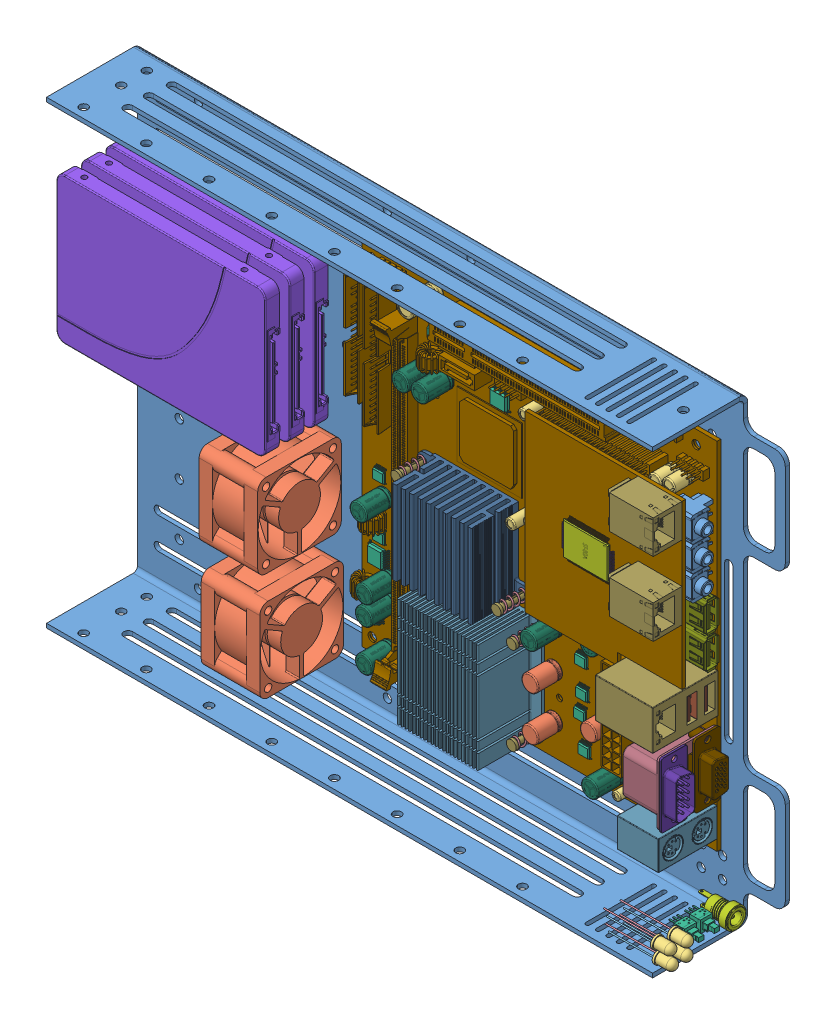
SolidWorks assembly kubebox_tray_itx, configuration Predeterminado. Lengths in mm.
Overall size (310 220 48.86).
125 component instances, 32 part files, 1 mates.
Components (placement in the parent):
- kubebox_tray-1: kubebox_tray [Predeterminado] at (-106.1016 -89.1854 250) size (310 220 45.5)
- Fan-40x40-1: Fan-40x40 [28mm] at (-84.3442 -51.7342 270.7277) x (0 0 -1) z (-1 0 0) size (48.86 43.8 28.03)
- LED 5mm green.step-2: LED 5mm green.step [Predeterminado] at (111.4078 -83.8857 281.3681) x (-0.004686 -0.000144 -0.999989) z (0.999988 0.001702 -0.004686) size (5.8 5.4 33.7)
  - F6rper 5mm.step-1: F6rper 5mm.step [Predeterminado] at origin size (5.8 5.4 8.7)
  - Anode.step-1: Anode.step [Predeterminado] at (0 1.27 -25) size (0.54 0.54 25)
  - Kadode.step-1: Kadode.step [Predeterminado] at (0 -1.27 -25) size (0.54 0.54 23.5)
- LED 5mm green.step-3: LED 5mm green.step [Predeterminado] at (111.773 -77.6908 281.5141) x (-0.004686 -0.000144 -0.999989) z (0.999988 0.001702 -0.004686) size (5.8 5.4 33.7)
  - F6rper 5mm.step-1: F6rper 5mm.step [Predeterminado] at origin size (5.8 5.4 8.7)
  - Anode.step-1: Anode.step [Predeterminado] at (0 1.27 -25) size (0.54 0.54 25)
  - Kadode.step-1: Kadode.step [Predeterminado] at (0 -1.27 -25) size (0.54 0.54 23.5)
- LED 5mm green.step-4: LED 5mm green.step [Predeterminado] at (111.6884 -83.9214 288.5994) x (-0.004686 -0.000144 -0.999989) z (0.999988 0.001702 -0.004686) size (5.8 5.4 33.7)
  - F6rper 5mm.step-1: F6rper 5mm.step [Predeterminado] at origin size (5.8 5.4 8.7)
  - Anode.step-1: Anode.step [Predeterminado] at (0 1.27 -25) size (0.54 0.54 25)
  - Kadode.step-1: Kadode.step [Predeterminado] at (0 -1.27 -25) size (0.54 0.54 23.5)
- LED 5mm green.step-5: LED 5mm green.step [Predeterminado] at (111.1 -77.7464 288.8261) x (-0.004686 -0.000144 -0.999989) z (0.999988 0.001702 -0.004686) size (5.8 5.4 33.7)
  - F6rper 5mm.step-1: F6rper 5mm.step [Predeterminado] at origin size (5.8 5.4 8.7)
  - Anode.step-1: Anode.step [Predeterminado] at (0 1.27 -25) size (0.54 0.54 25)
  - Kadode.step-1: Kadode.step [Predeterminado] at (0 -1.27 -25) size (0.54 0.54 23.5)
- Toggle Button (6 x 6 x 10mm) - NON Latching.stp-1: Toggle Button (6 x 6 x 10mm) - NON Latching.stp [Predeterminado] at (107.7716 -80.5751 266.7149) x (0 1 0) z (1 0 0) size (5.74 5.82 13.39)
- Toggle Button (6 x 6 x 10mm) - NON Latching.stp-2: Toggle Button (6 x 6 x 10mm) - NON Latching.stp [Predeterminado] at (107.7786 -80.552 274.244) x (0 1 0) z (1 0 0) size (5.74 5.82 13.39)
- Fan-40x40-2: Fan-40x40 [28mm] at (-85.3503 -0.9212 270.7277) x (0 0 -1) z (-1 0 0) size (48.86 43.8 28.03)
- 2.1mm x 5.5mm Round Chasis Female Socket DC Connector Jack-1: 2.1mm x 5.5mm Round Chasis Female Socket DC Connector Jack [Default] at (113.9605 -80.8969 257.09) x (0 0 -1) z (1 0 0) size (10 10 17.7)
- Standard 520 model-1: Standard 520 model [Default] at (-125.8554 63.2761 262.1971) x (0 1 0) z (1 0 0) size (69.85 7 100.3)
- Standard 520 model-2: Standard 520 model [Default] at (-125.8457 63.2851 273.7903) x (0 1 0) z (1 0 0) size (69.85 7 100.3)
- Standard 520 model-3: Standard 520 model [Default] at (-125.8434 63.2833 285.5347) x (0 1 0) z (1 0 0) size (69.85 7 100.3)
- Motherboard-1: Motherboard [Default] at (24.0384 27.9346 255.9838) x (0 1 0) z (1 0 0) size (170 37.23 177.79)
  - Motherboard-Mini-ITX-1: Motherboard-Mini-ITX [Default] at origin size (170 18.6 170)
  - User Library-TS-65259-ZH-1: User Library-TS-65259-ZH [Default] at (-7.4545 1.8 -30) x (0 0 -1) z (1 0 0) size (54 24.6 40.05)
    - User Library-TS-65259-ZH_BGA Heat Sink-2: User Library-TS-65259-ZH_BGA Heat Sink [Default] at origin size (54 22.5 40.05)
    - User Library-TS-65259-ZH_T710 Material-1: User Library-TS-65259-ZH_T710 Material [Default] x (1 0 0) z (0 -1 0) size (31.75 31.75 0.2)
    - User Library-TS-65259-ZH_Brass Pin-1: User Library-TS-65259-ZH_Brass Pin [Default] at (-24 14.77 -15.7) size (4.7 16.87 4.7)
    - User Library-TS-65259-ZH_Spring-Uncompressed-1: User Library-TS-65259-ZH_Spring-Uncompressed [Default] at (-24 14.3143 -15.7) x (1 0 0) z (0 -1 0) size (5.34 6 13)
    - User Library-TS-65259-ZH_Brass Pin-2: User Library-TS-65259-ZH_Brass Pin [Default] at (24 14.77 15.7) size (4.7 16.87 4.7)
    - User Library-TS-65259-ZH_Spring-Uncompressed-2: User Library-TS-65259-ZH_Spring-Uncompressed [Default] at (24 0.7057 15.7) x (1 0 0) z (0 1 0) size (5.34 6 13)
  - Heat Sink A-1: Heat Sink A [Default] at (-56.3 1.8 -22.5) x (0 0 -1) z (1 0 0) size (50 26.5 52)
  - User Library-TS-65259-ZH_Brass Pin-1: User Library-TS-65259-ZH_Brass Pin [Default] at (-35.3 14.77 -44.5) x (0 0 -1) z (1 0 0) size (4.7 16.87 4.7)
  - User Library-TS-65259-ZH_Spring-Uncompressed-1: User Library-TS-65259-ZH_Spring-Uncompressed [Default] at (-35.3 0.8156 -44.5) x (0.439893 0 -0.89805) z (0 1 0) size (5.34 6 13)
  - User Library-CAPACITOR-2-1: User Library-CAPACITOR-2 [D=8] at (-79.4531 -4.5974 -71.4991) size (8.26 14.29 8.25)
  - User Library-CAPACITOR-2-2: User Library-CAPACITOR-2 [D=8] at (-50.3757 -4.5974 -71.4991) size (8.26 14.29 8.25)
  - User Library-CAPACITOR-2-3: User Library-CAPACITOR-2 [D=8] at (-17.5304 -4.5974 -74.0227) size (8.26 14.29 8.25)
  - User Library-CAPACITOR-2-4: User Library-CAPACITOR-2 [D=8] at (-59.6152 -4.5974 -71.4991) size (8.26 14.29 8.25)
  - User Library-CAPACITOR-2-5: User Library-CAPACITOR-2 [D=8] at (46.2267 -4.5974 -44.8893) x (-0.064546 0 -0.997915) z (0.997915 0 -0.064546) size (8.26 14.29 8.25)
  - User Library-CAPACITOR-2-6: User Library-CAPACITOR-2 [D=8] at (46.2268 -4.5974 -54.0316) size (8.26 14.29 8.25)
  - User Library-CAPACITOR-2-7: User Library-CAPACITOR-2 [D=8] at (-18.1774 -4.5974 36.0078) x (-0.064546 0 -0.997915) z (0.997915 0 -0.064546) size (8.26 14.29 8.25)
  - User Library-CAPACITOR-2-8: User Library-CAPACITOR-2 [D=8] at (9.1349 -4.5974 42.427) x (-0.064546 0 -0.997915) z (0.997915 0 -0.064546) size (8.26 14.29 8.25)
  - User Library-CAPACITOR-2-9: User Library-CAPACITOR-2 [D=8] at (53.4161 -4.5974 31.2418) x (-0.064546 0 -0.997915) z (0.997915 0 -0.064546) size (8.26 14.29 8.25)
  - User Library-CAPACITOR-2-10: User Library-CAPACITOR-2 [D=8] at (27.2615 -4.5974 57.1967) x (-0.064546 0 -0.997915) z (0.997915 0 -0.064546) size (8.26 14.29 8.25)
  - User Library-CAPACITOR-2-11: User Library-CAPACITOR-2 [D=8] at (17.5542 -4.5974 22.737) x (-0.064546 0 -0.997915) z (0.997915 0 -0.064546) size (8.26 14.29 8.25)
  - User Library-CAPACITOR-2-12: User Library-CAPACITOR-2 [D=8] at (-76.824 -4.5974 36.7263) x (-0.064546 0 -0.997915) z (0.997915 0 -0.064546) size (8.26 14.29 8.25)
  - User Library-USB Socket-1: User Library-USB Socket [Default] at (14.3 1.8 78.48) size (14.6 8.03 14.23)
  - User Library-USB Socket-2: User Library-USB Socket [Default] at (-1.1 1.8 78.48) size (14.6 8.03 14.23)
  - User Library-DB15HD-1: User Library-DB15HD [Predeterminado] at (-47.5 23.6419 85.4) size (31 12.5 18)
  - User Library-DB15recept_straight-1: User Library-DB15recept_straight [Default] at (-47.5 7.6681 86.3906) size (30.81 12.55 17.86)
  - CUI-SJ1-3545N-1: CUI-SJ1-3545N [Pink] at (54 9.8 88.5) x (0 0 1) z (0 1 0) size (15 12.2 16.5)
  - SW3DPS-ELECTROLITIC CAPACITOR RADIAL 8X12-DEFAULT-1: SW3DPS-ELECTROLITIC CAPACITOR RADIAL 8X12-DEFAULT [Default] at (-69.4896 1.8 7.3403) x (0.957319 0 0.289034) z (-0.289034 0 0.957319) size (8 14.5 8)
  - User Library-Capacitor Radial Electrolitic-1: User Library-Capacitor Radial Electrolitic [CAPPR350-800X1500] at (79.996 1.8 -49.5016) x (0.219712 0 -0.975565) z (0.975565 0 0.219712) size (8.01 17.73 8)
  - User Library-QFP-24P400X400LS050h120-1: User Library-QFP-24P400X400LS050h120 [Default] at (-16.4 2.9831 53.4) x (0 0 -1) z (0 1 0) size (10.8 10.8 2.16)
  - User Library-so14p865x390ll600ls127h155-1: User Library-so14p865x390ll600ls127h155 [1] at (16.7443 1.8 54.05) x (0 0 -1) z (0 1 0) size (6 6.07 1.55)
  - User Library-ssop16p500x440ls065h200-1: User Library-ssop16p500x440ls065h200 [Default] at (70.8 1.8 -47) x (1 0 0) z (0 1 0) size (6.4 5 2)
  - User Library-ST-80A-1: User Library-ST-80A [Default] at (2.5646 1.3604 55.1237) size (15.56 1.47 21.26)
    - User Library-ST-80A_ST-80A_Body-1: User Library-ST-80A_ST-80A_Body [Default] at (1.4361 0.5396 -1.1244) size (12 1.4 12)
    - User Library-ST-80A_Pin-9: User Library-ST-80A_Pin [1] at (-3.4851 0.946 5.8923) x (0 0 1) z (-1 0 0) size (1.78 0.97 9.91)
    - User Library-ST-80A_Pin1-9: User Library-ST-80A_Pin1 [Default] at (8.4529 0.946 4.2147) size (1.78 0.97 19.05)
    - User Library-ST-80A_Pin1-10: User Library-ST-80A_Pin1 [Default] at (-5.5806 0.946 -14.3781) x (-1 0 0) z (0 0 -1) size (1.78 0.97 19.05)
    - User Library-ST-80A_Pin-11: User Library-ST-80A_Pin [1] at (5.9383 0.946 -8.1412) x (0 0 -1) z (1 0 0) size (1.78 0.97 9.91)
    - User Library-ST-80A_Pin-12: User Library-ST-80A_Pin [1] at (-5.5806 0.946 -6.296) x (-1 0 0) z (0 0 -1) size (1.78 0.97 9.91)
    - User Library-ST-80A_Pin-13: User Library-ST-80A_Pin [1] at (8.4529 0.946 3.1528) size (1.78 0.97 9.91)
  - User Library-tsop24p600x1640ls050h120-1: User Library-tsop24p600x1640ls050h120 [Default] at (-11 2 14.8) x (0 0 -1) z (0 1 0) size (18 6 1.2)
  - User Library-Capacitor Radial Electrolitic-2: User Library-Capacitor Radial Electrolitic [CAPPR200-500X1100] at (-43.7308 1.8 -20.0233) size (5.01 13.73 5)
  - User Library-ssop16p500x440ls065h200-2: User Library-ssop16p500x440ls065h200 [1] at (-42.25 2.3907 -76.2) x (0 0 1) z (0 1 0) size (9.6 7.5 3)
  - User Library-ST-80A-2: User Library-ST-80A [1] at (30.2619 1.2704 34.3205) size (19.16 1.47 25.16)
    - User Library-ST-80A_ST-80A_Body-1: User Library-ST-80A_ST-80A_Body [1] at (1.4361 0.5396 -1.1244) size (15.6 1.4 21.6)
    - User Library-ST-80A_Pin-9: User Library-ST-80A_Pin [1] at (-2.9793 0.946 10.6955) x (0 0 1) z (-1 0 0) size (1.78 0.97 9.91)
    - User Library-ST-80A_Pin1-9: User Library-ST-80A_Pin1 [Default] at (10.2541 0.946 8.6715) size (1.78 0.97 19.05)
    - User Library-ST-80A_Pin1-10: User Library-ST-80A_Pin1 [Default] at (-7.3799 0.946 -9.9213) x (-1 0 0) z (0 0 -1) size (1.78 0.97 19.05)
    - User Library-ST-80A_Pin-11: User Library-ST-80A_Pin [1] at (6.4695 0.946 -12.9392) x (0 0 -1) z (1 0 0) size (1.78 0.97 9.91)
    - User Library-ST-80A_Pin-12: User Library-ST-80A_Pin [1] at (-5.5806 0.946 -6.296) x (-1 0 0) z (0 0 -1) size (1.78 0.97 9.91)
    - User Library-ST-80A_Pin-13: User Library-ST-80A_Pin [1] at (8.4529 0.946 3.1528) size (1.78 0.97 9.91)
  - User Library-ssop16p500x440ls065h200-3: User Library-ssop16p500x440ls065h200 [Default] at (-36.8 2.4 61.5) x (1 0 0) z (0 1 0) size (6.4 5 2)
  - SW3DPS-ELECTROLITIC CAPACITOR RADIAL 8X12-DEFAULT-2: SW3DPS-ELECTROLITIC CAPACITOR RADIAL 8X12-DEFAULT [Default] at (-54.5523 1.8 35.2905) x (0.957319 0 0.289034) z (-0.289034 0 0.957319) size (8 14.5 8)
  - SW3DPS-ELECTROLITIC CAPACITOR RADIAL 8X12-DEFAULT-3: SW3DPS-ELECTROLITIC CAPACITOR RADIAL 8X12-DEFAULT [Default] at (-48.2292 1.8 7.3403) x (0.957319 0 0.289034) z (-0.289034 0 0.957319) size (8 14.5 8)
  - User Library-TS-65259-ZH_Brass Pin-2: User Library-TS-65259-ZH_Brass Pin [Default] at (-77.3 14.77 -44.5) x (0.837243 0 0.546832) z (-0.546832 0 0.837243) size (4.7 16.87 4.7)
  - User Library-TS-65259-ZH_Brass Pin-3: User Library-TS-65259-ZH_Brass Pin [Default] at (-77.3 14.77 -0.5) x (0 0 -1) z (1 0 0) size (4.7 16.87 4.7)
  - User Library-TS-65259-ZH_Brass Pin-4: User Library-TS-65259-ZH_Brass Pin [Default] at (-35.3 14.77 -0.5) x (0.837243 0 0.546832) z (-0.546832 0 0.837243) size (4.7 16.87 4.7)
  - User Library-TS-65259-ZH_Spring-Uncompressed-2: User Library-TS-65259-ZH_Spring-Uncompressed [Default] at (-35.3 0.8156 -0.5) x (-0.772723 0 0.634744) z (0 1 0) size (5.34 6 13)
  - User Library-TS-65259-ZH_Spring-Uncompressed-3: User Library-TS-65259-ZH_Spring-Uncompressed [Default] at (-77.3 0.8156 -44.5) x (0.999805 0 0.01976) z (0 1 0) size (5.34 6 13)
  - User Library-TS-65259-ZH_Spring-Uncompressed-4: User Library-TS-65259-ZH_Spring-Uncompressed [Default] at (-77.3 0.8156 -0.5) x (-0.998104 0 0.061542) z (0 1 0) size (5.34 6 13)
  - CUI-SJ1-3545N-2: CUI-SJ1-3545N [Green] at (41.8 9.8 88.5) x (0 0 1) z (0 1 0) size (15 12.2 16.5)
  - CUI-SJ1-3545N-3: CUI-SJ1-3545N [Blue] at (29.6 9.8 88.5) x (0 0 1) z (0 1 0) size (15 12.2 16.5)
  - User Library-Capacitor Radial Electrolitic-4: User Library-Capacitor Radial Electrolitic [CAPPR250-630X980] at (64.5347 1.81 71.4955) x (0.219712 0 -0.975565) z (0.975565 0 0.219712) size (6.31 12.53 6.3)
  - User Library-Capacitor Radial Electrolitic-5: User Library-Capacitor Radial Electrolitic [CAPPR250-630X1500] at (41.4632 1.81 58.7461) x (0.219712 0 -0.975565) z (0.975565 0 0.219712) size (6.31 17.73 6.3)
  - User Library-Capacitor Radial Electrolitic-6: User Library-Capacitor Radial Electrolitic [CAPPR200-500X1150] at (41.4632 1.81 52.1875) x (0.219712 0 -0.975565) z (0.975565 0 0.219712) size (5.01 14.23 5)
  - User Library-Capacitor Radial Electrolitic-7: User Library-Capacitor Radial Electrolitic [CAPPR250-630X980] at (63.1844 1.81 64.8938) x (0.219712 0 -0.975565) z (0.975565 0 0.219712) size (6.31 12.53 6.3)
  - Samtec-USB-A-D-S-B-VU-1: Samtec-USB-A-D-S-B-VU [Default] at (-19.2 2.9 76.495) size (15.8 19.67 17.65)
  - User Library-RJ45-8P-Pipe-Cat6-1: User Library-RJ45-8P-Pipe-Cat6 [Default] at (-19.2 18.4 64.2) size (21.35 33.02 27.5)
  - User Library-ssop16p500x440ls065h200-4: User Library-ssop16p500x440ls065h200 [Default] at (62.8 1.8 -49.5) x (1 0 0) z (0 1 0) size (6.4 5 2)
  - User Library-ssop16p500x440ls065h200-5: User Library-ssop16p500x440ls065h200 [Default] at (-49.8 2.6 22.5) x (1 0 0) z (0 1 0) size (6.4 5 2)
  - User Library-ssop16p500x440ls065h200-6: User Library-ssop16p500x440ls065h200 [Default] at (-72.8 2.6 23.5) x (1 0 0) z (0 1 0) size (6.4 5 2)
  - User Library-ssop16p500x440ls065h200-7: User Library-ssop16p500x440ls065h200 [Default] at (-36.3 2.6 22) x (1 0 0) z (0 1 0) size (6.4 5 2)
  - User Library-ssop16p500x440ls065h200-8: User Library-ssop16p500x440ls065h200 [Default] at (-58.8 2.6 21.5) x (1 0 0) z (0 1 0) size (6.4 5 2)
  - User Library-ssop16p500x440ls065h200-9: User Library-ssop16p500x440ls065h200 [Default] at (16.7 2.6 13) x (1 0 0) z (0 1 0) size (6.4 5 2)
  - User Library-so14p865x390ll600ls127h155-2: User Library-so14p865x390ll600ls127h155 [1] at (33.8028 1.8 55.0746) x (0 0 -1) z (0 1 0) size (6 6.07 1.55)
  - User Library-ssop16p500x440ls065h200-10: User Library-ssop16p500x440ls065h200 [Default] at (51.3 2.6 56.9) x (1 0 0) z (0 1 0) size (6.4 5 2)
  - User Library-ssop16p500x440ls065h200-11: User Library-ssop16p500x440ls065h200 [1] at (52.2 2.3907 -17.25) x (1 0 0) z (0 1 0) size (9.6 7.5 3)
  - User Library-ssop16p500x440ls065h200-12: User Library-ssop16p500x440ls065h200 [Default] at (-8.7786 1.8 -75.5) x (1 0 0) z (0 1 0) size (6.4 5 2)
  - User Library-ssop16p500x440ls065h200-13: User Library-ssop16p500x440ls065h200 [Default] at (-34.0566 1.8 -75.5) x (1 0 0) z (0 1 0) size (6.4 5 2)
  - User Library-ssop16p500x440ls065h200-14: User Library-ssop16p500x440ls065h200 [1] at (-66.75 2.3907 -79) x (0 0 1) z (0 1 0) size (9.6 7.5 3)
  - User Library-Capacitor Radial Electrolitic-8: User Library-Capacitor Radial Electrolitic [CAPPR200-500X1150] at (17.2298 1.81 6.0657) x (0.219712 0 -0.975565) z (0.975565 0 0.219712) size (5.01 14.23 5)
  - User Library-Capacitor Radial Electrolitic-9: User Library-Capacitor Radial Electrolitic [CAPPR200-500X1150] at (12.4626 1.81 -2.6529) x (0.219712 0 -0.975565) z (0.975565 0 0.219712) size (5.01 14.23 5)
  - User Library-CAPACITOR-2-13: User Library-CAPACITOR-2 [D=8] at (-30.2607 -4.5974 7.2973) x (-0.064546 0 -0.997915) z (0.997915 0 -0.064546) size (8.26 14.29 8.25)
  - User Library-Capacitor Radial Electrolitic-10: User Library-Capacitor Radial Electrolitic [CAPPR200-500X1150] at (60.8999 1.81 3.545) x (0.219712 0 -0.975565) z (0.975565 0 0.219712) size (5.01 14.23 5)
  - User Library-Capacitor Radial Electrolitic-11: User Library-Capacitor Radial Electrolitic [CAPPR150-400X700] at (7.4823 1.8 68.8681) x (0.219712 0 -0.975565) z (0.975565 0 0.219712) size (4.01 9.73 4)
  - User Library-Capacitor Radial Electrolitic-12: User Library-Capacitor Radial Electrolitic [CAPPR150-400X700] at (-79.4532 1.81 43.5549) x (0.219712 0 -0.975565) z (0.975565 0 0.219712) size (4.01 9.73 4)
  - Monitor connector Housing-1: Monitor connector Housing [Default] at (-47.5 23.6419 85.4) size (30.5 28.3 17.81)
  - User Library-ST-80A-3: User Library-ST-80A [1] at (24.7839 18.1404 41.3205) size (19.16 1.47 25.16)
    - User Library-ST-80A_ST-80A_Body-1: User Library-ST-80A_ST-80A_Body [1] at (1.4361 0.5396 -1.1244) size (15.6 1.4 21.6)
    - User Library-ST-80A_Pin-9: User Library-ST-80A_Pin [1] at (-2.9793 0.946 10.6955) x (0 0 1) z (-1 0 0) size (1.78 0.97 9.91)
    - User Library-ST-80A_Pin1-9: User Library-ST-80A_Pin1 [Default] at (10.2541 0.946 8.6715) size (1.78 0.97 19.05)
    - User Library-ST-80A_Pin1-10: User Library-ST-80A_Pin1 [Default] at (-7.3799 0.946 -9.9213) x (-1 0 0) z (0 0 -1) size (1.78 0.97 19.05)
    - User Library-ST-80A_Pin-11: User Library-ST-80A_Pin [1] at (6.4695 0.946 -12.9392) x (0 0 -1) z (1 0 0) size (1.78 0.97 9.91)
    - User Library-ST-80A_Pin-12: User Library-ST-80A_Pin [1] at (-5.5806 0.946 -6.296) x (-1 0 0) z (0 0 -1) size (1.78 0.97 9.91)
    - User Library-ST-80A_Pin-13: User Library-ST-80A_Pin [1] at (8.4529 0.946 3.1528) size (1.78 0.97 9.91)
  - User Library-RJ45-8P-Pipe-Cat6-2: User Library-RJ45-8P-Pipe-Cat6 [Single Lan] at (25.3 18.6 64) size (21.35 21.42 24)
  - User Library-PS2-2-1: User Library-PS2-2 [Clavier] at (-73 8.8 67.9191) size (14 28 19.8)
  - User Library-RJ45-8P-Pipe-Cat6-3: User Library-RJ45-8P-Pipe-Cat6 [Single Lan] at (60.5 18.6 64) size (21.35 21.42 24)
Mates (geometry in assembly coordinates):
- Concentric2: concentric aligned: cylinder of kubebox_tray-1 through (76.0384 -50.6654 248) axis (0 0 1) radius 2; cylinder of Motherboard-1/Motherboard-Mini-ITX-1 through (76.0384 -50.6654 255.9838) axis (0 0 1) radius 2
